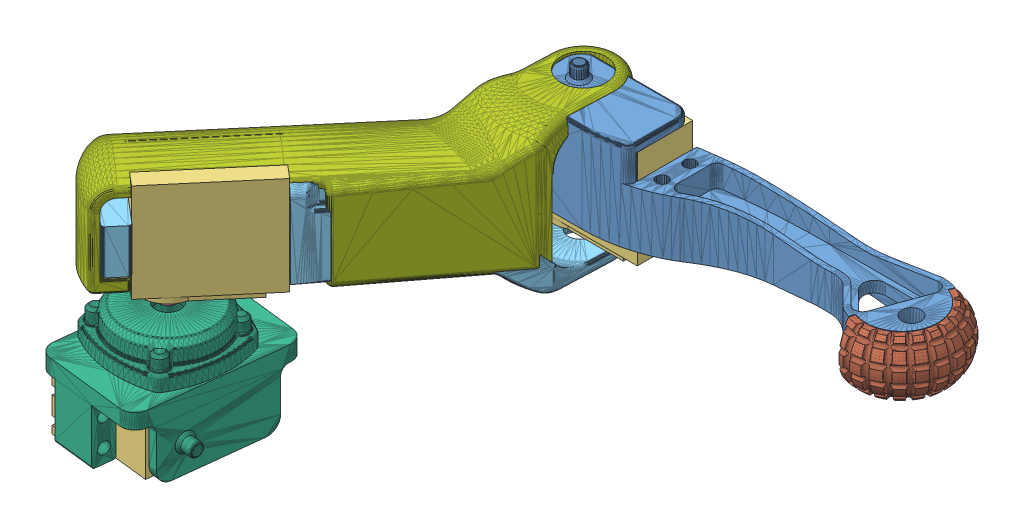
SolidWorks assembly right_foot_front, configuration Default. Lengths in mm.
Overall size (236.52 96.4 141.61).
14 component instances, 7 part files, 20 mates.
Components (placement in the parent):
- R_wrist_mg-1: R_wrist_mg [Default] at (-88.5645 -25.7472 139.9903) size (149.99 36.9 30)
- foot-1: foot [Default] at (37.4355 -5.9472 149.9903) x (0.342021 0 -0.939692) z (-0.939692 0 -0.342021) size (38.32 20 19.41)
- MG996R-1: MG996R [Default] at (-68.3145 3.2528 149.9903) x (1 0 0) z (0 0 -1) size (54.5 43 20)
  - servo-1: servo [Default] at origin size (54.5 39 20)
  - shaft-1: shaft [Default] at (-10.1089 43 0) x (-0.837169 0 -0.546944) z (-0.546944 0 0.837169) size (5.9 19.57 5.9)
- R_arm_mg-1: R_arm_mg [Default] at (-151.1073 -85.7472 241.8085) x (0.762308 0 0.647215) z (0.647215 0 -0.762308) size (38.24 39.8 137.4)
- MG996R-2: MG996R [Default] at (-130.3782 -3.7472 232.8439) x (0.647215 0 -0.762308) z (-0.762308 0 -0.647215) size (54.5 43 20)
  - servo-1: servo [Default] at origin size (54.5 39 20)
  - shaft-1: shaft [Default] at (-10.1089 43 0) x (-0.837169 0 -0.546944) z (-0.546944 0 0.837169) size (5.9 19.57 5.9)
- R_arm_joint_mg-1: R_arm_joint_mg [Default] at (-129.0263 -115.2472 261.8291) x (0 -1 0) z (0.113077 0 -0.993586) size (37.5 46 56.5)
- R_arm_cover-1: R_arm_cover [Default] at (-161.6944 -48.0472 242.0025) x (0.762308 0 0.647215) z (0.647215 0 -0.762308) size (41.16 45 143.55)
- MG996R-3: MG996R [Default] at (-120.775 -75.2472 242.3875) x (0.113077 0 -0.993586) z (0 1 0) size (54.5 43 20)
  - servo-1: servo [Default] at origin size (54.5 39 20)
  - shaft-1: shaft [Default] at (-10.1089 43 0) x (-0.837169 0 -0.546944) z (-0.546944 0 0.837169) size (5.9 19.57 5.9)
Mates (geometry in assembly coordinates):
- Coincident1: coincident anti-aligned: plane of R_wrist_mg-1 through (25.9102 -25.7472 181.6558) normal (0.939692 0 0.342021); plane of foot-1 through (37.4355 -5.9472 149.9903) normal (-0.939692 0 -0.342021)
- Coincident2: coincident anti-aligned: plane of R_wrist_mg-1 through (-88.5645 -8.7472 139.9903) normal (0 1 0); plane of foot-1 through (37.4355 -8.7472 149.9903) normal (0 -1 0)
- Coincident4: coincident: plane of R_wrist_mg-1 through (-84.7772 -25.7472 127.2361) normal (-0.284661 0 0.958628); point of foot-1
- Coincident5: coincident anti-aligned: plane of R_wrist_mg-1 through (-88.5645 3.2528 139.9903) normal (0 -1 0); plane of MG996R-1/servo-1 through (-68.3145 3.2528 149.9903) normal (0 1 0)
- Coincident6: coincident anti-aligned: plane of R_wrist_mg-1 through (-88.5645 -25.7472 139.9903) normal (1 0 0); plane of MG996R-1/servo-1 through (-88.5645 -32.2472 139.9903) normal (-1 0 0)
- Coincident7: coincident anti-aligned: plane of R_wrist_mg-1 through (-88.5645 -25.7472 159.9903) normal (0 0 -1); plane of MG996R-1/servo-1 through (-88.5645 -32.2472 159.9903) normal (0 0 1)
- Parallel1: parallel anti-aligned: plane of R_wrist_mg-1 through (-88.5645 6.1528 139.9903) normal (0 1 0); plane of R_arm_mg-1 through (-151.1073 -45.7472 241.8085) normal (0 -1 0)
- Coincident9: coincident: line of MG996R-1/shaft-1 through (-78.4234 -39.7472 149.9903) axis (0 1 0)
- Distance1: distance = 1 mm anti-aligned: plane of MG996R-1/shaft-1 through (-78.4234 -39.7472 149.9903) normal (0 -1 0); plane of R_arm_mg-1 through (-151.1073 -40.7472 241.8085) normal (0 1 0)
- Coincident11: coincident anti-aligned: plane of R_arm_mg-1 through (-151.1073 -30.7472 241.8085) normal (0 -1 0); plane of MG996R-2/servo-1 through (-142.614 -30.7472 254.5947) normal (0 1 0)
- Coincident12: coincident anti-aligned: plane of R_arm_mg-1 through (-124.8951 -85.7472 210.935) normal (-0.647215 0 0.762308); plane of MG996R-2/servo-1 through (-124.8951 -39.2472 210.935) normal (0.647215 0 -0.762308)
- Coincident13: coincident anti-aligned: plane of R_arm_mg-1 through (-151.1073 -85.7472 241.8085) normal (0.762308 0 0.647215); plane of MG996R-2/servo-1 through (-151.1073 -39.2472 241.8085) normal (-0.762308 0 -0.647215)
- Distance3: distance = 1 mm anti-aligned: plane of R_arm_joint_mg-1 through (-129.0263 -47.7472 261.8291) normal (0 1 0); plane of MG996R-2/shaft-1 through (-136.9208 -46.7472 240.55) normal (0 -1 0)
- Coincident17: coincident: line of MG996R-2/shaft-1 through (-136.9208 -46.7472 240.55) axis (0 1 0)
- Coincident20: coincident anti-aligned: plane of R_arm_cover-1 through (-162.3416 -48.0472 242.7648) normal (0.647215 0 -0.762308); plane of R_arm_mg-1 through (-156.2851 -85.7472 247.9069) normal (-0.647215 0 0.762308)
- Coincident21: coincident anti-aligned: plane of MG996R-2/servo-1 through (-142.614 -33.2472 254.5947) normal (0 -1 0); plane of R_arm_cover-1 through (-161.6944 -33.2472 242.0025) normal (0 1 0)
- Coincident22: coincident aligned: plane of MG996R-2/servo-1 through (-136.6235 -30.7472 254.1055) normal (0.762308 0 0.647215); plane of R_arm_cover-1 through (-141.154 -48.0472 259.4417) normal (0.762308 0 0.647215)
- Coincident23: coincident anti-aligned: plane of R_arm_joint_mg-1 through (-149.8916 -115.2472 259.4545) normal (-0.993586 0 -0.113077); plane of MG996R-3/servo-1 through (-150.3722 -79.9972 263.6773) normal (0.993586 0 0.113077)
- Coincident24: coincident anti-aligned: plane of R_arm_joint_mg-1 through (-129.0263 -65.2472 261.8291) normal (0 -1 0); plane of MG996R-3/servo-1 through (-158.3371 -65.2472 258.4934) normal (0 1 0)
- Coincident25: coincident anti-aligned: plane of R_arm_joint_mg-1 through (-129.0263 -115.2472 261.8291) normal (0.113077 0 -0.993586); plane of MG996R-3/servo-1 through (-158.3371 -65.2472 258.4934) normal (-0.113077 0 0.993586)
